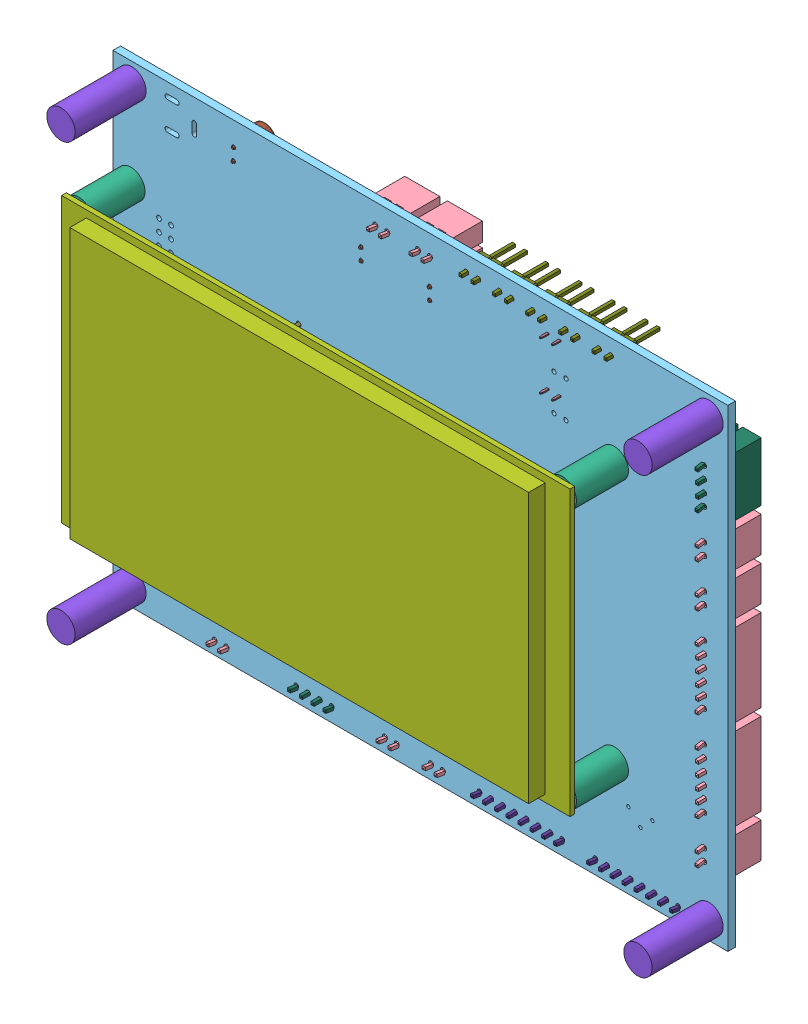
SolidWorks assembly MCU, configuration 默认. Lengths in mm. (continued)
Components (placement in the parent): (continued)
- MCU(2)^MCU-1: MCU(2)^MCU [默认] at origin size (130 100 11.94) (virtual) (continued)
  - R_0805^MCU(2)_MCU-76: R_0805^MCU(2)_MCU [默认] at (107.6 84.5 -0.05) x (1 0 0) z (0 0 -1) size (2 1.25 0.5) (virtual)
    - SOLID-1^R_0805_MCU(2)_MCU-1: SOLID-1^R_0805_MCU(2)_MCU [默认] at origin size (2 1.25 0.5) (virtual)
  - R_0805^MCU(2)_MCU-77: R_0805^MCU(2)_MCU [默认] at (120 86.5 -0.05) x (-1 0 0) z (0 0 -1) size (2 1.25 0.5) (virtual)
    - SOLID-1^R_0805_MCU(2)_MCU-1: SOLID-1^R_0805_MCU(2)_MCU [默认] at origin size (2 1.25 0.5) (virtual)
  - R_0805^MCU(2)_MCU-78: R_0805^MCU(2)_MCU [默认] at (51.9 8.7 -0.05) x (-1 0 0) z (0 0 -1) size (2 1.25 0.5) (virtual)
    - SOLID-1^R_0805_MCU(2)_MCU-1: SOLID-1^R_0805_MCU(2)_MCU [默认] at origin size (2 1.25 0.5) (virtual)
  - R_0805^MCU(2)_MCU-79: R_0805^MCU(2)_MCU [默认] at (46.929 55.357 -0.05) x (0.707107 0.707107 0) z (0 0 -1) size (2 1.25 0.5) (virtual)
    - SOLID-1^R_0805_MCU(2)_MCU-1: SOLID-1^R_0805_MCU(2)_MCU [默认] at origin size (2 1.25 0.5) (virtual)
  - R_0805^MCU(2)_MCU-80: R_0805^MCU(2)_MCU [默认] at (99.5 8.5 -0.05) x (-1 0 0) z (0 0 -1) size (2 1.25 0.5) (virtual)
    - SOLID-1^R_0805_MCU(2)_MCU-1: SOLID-1^R_0805_MCU(2)_MCU [默认] at origin size (2 1.25 0.5) (virtual)
  - R_0805^MCU(2)_MCU-81: R_0805^MCU(2)_MCU [默认] at (103.05 8.5 -0.05) x (-1 0 0) z (0 0 -1) size (2 1.25 0.5) (virtual)
    - SOLID-1^R_0805_MCU(2)_MCU-1: SOLID-1^R_0805_MCU(2)_MCU [默认] at origin size (2 1.25 0.5) (virtual)
  - R_0805^MCU(2)_MCU-82: R_0805^MCU(2)_MCU [默认] at (106.5 8.5 -0.05) x (1 0 0) z (0 0 -1) size (2 1.25 0.5) (virtual)
    - SOLID-1^R_0805_MCU(2)_MCU-1: SOLID-1^R_0805_MCU(2)_MCU [默认] at origin size (2 1.25 0.5) (virtual)
  - R_0805^MCU(2)_MCU-83: R_0805^MCU(2)_MCU [默认] at (110 8.5 -0.05) x (1 0 0) z (0 0 -1) size (2 1.25 0.5) (virtual)
    - SOLID-1^R_0805_MCU(2)_MCU-1: SOLID-1^R_0805_MCU(2)_MCU [默认] at origin size (2 1.25 0.5) (virtual)
  - R_0805^MCU(2)_MCU-84: R_0805^MCU(2)_MCU [默认] at (113.5 8.5 -0.05) x (-1 0 0) z (0 0 -1) size (2 1.25 0.5) (virtual)
    - SOLID-1^R_0805_MCU(2)_MCU-1: SOLID-1^R_0805_MCU(2)_MCU [默认] at origin size (2 1.25 0.5) (virtual)
  - R_0805^MCU(2)_MCU-85: R_0805^MCU(2)_MCU [默认] at (117 8.5 -0.05) x (-1 0 0) z (0 0 -1) size (2 1.25 0.5) (virtual)
    - SOLID-1^R_0805_MCU(2)_MCU-1: SOLID-1^R_0805_MCU(2)_MCU [默认] at origin size (2 1.25 0.5) (virtual)
  - R_0805^MCU(2)_MCU-86: R_0805^MCU(2)_MCU [默认] at (76.5 8.5 -0.05) x (1 0 0) z (0 0 -1) size (2 1.25 0.5) (virtual)
    - SOLID-1^R_0805_MCU(2)_MCU-1: SOLID-1^R_0805_MCU(2)_MCU [默认] at origin size (2 1.25 0.5) (virtual)
  - R_0805^MCU(2)_MCU-87: R_0805^MCU(2)_MCU [默认] at (80 8.5 -0.05) x (1 0 0) z (0 0 -1) size (2 1.25 0.5) (virtual)
    - SOLID-1^R_0805_MCU(2)_MCU-1: SOLID-1^R_0805_MCU(2)_MCU [默认] at origin size (2 1.25 0.5) (virtual)
  - R_0805^MCU(2)_MCU-88: R_0805^MCU(2)_MCU [默认] at (83.5 8.5 -0.05) x (1 0 0) z (0 0 -1) size (2 1.25 0.5) (virtual)
    - SOLID-1^R_0805_MCU(2)_MCU-1: SOLID-1^R_0805_MCU(2)_MCU [默认] at origin size (2 1.25 0.5) (virtual)
  - R_0805^MCU(2)_MCU-89: R_0805^MCU(2)_MCU [默认] at (87 8.5 -0.05) x (1 0 0) z (0 0 -1) size (2 1.25 0.5) (virtual)
    - SOLID-1^R_0805_MCU(2)_MCU-1: SOLID-1^R_0805_MCU(2)_MCU [默认] at origin size (2 1.25 0.5) (virtual)
  - R_0805^MCU(2)_MCU-90: R_0805^MCU(2)_MCU [默认] at (90.5 8.5 -0.05) x (1 0 0) z (0 0 -1) size (2 1.25 0.5) (virtual)
    - SOLID-1^R_0805_MCU(2)_MCU-1: SOLID-1^R_0805_MCU(2)_MCU [默认] at origin size (2 1.25 0.5) (virtual)
  - R_0805^MCU(2)_MCU-91: R_0805^MCU(2)_MCU [默认] at (94 8.5 -0.05) x (1 0 0) z (0 0 -1) size (2 1.25 0.5) (virtual)
    - SOLID-1^R_0805_MCU(2)_MCU-1: SOLID-1^R_0805_MCU(2)_MCU [默认] at origin size (2 1.25 0.5) (virtual)
  - SOT-23^MCU(2)_MCU-4: SOT-23^MCU(2)_MCU [默认] at (95.75 58.25 -0.05) x (0 1 0) z (0 0 -1) size (2.5 3 1.2) (virtual)
    - SOLID-4^SOT-23_MCU(2)_MCU-1: SOLID-4^SOT-23_MCU(2)_MCU [默认] at origin size (2.5 3 1.2) (virtual)
  - SOT-23^MCU(2)_MCU-5: SOT-23^MCU(2)_MCU [默认] at (99.75 53.35 -0.05) x (0 -1 0) z (0 0 -1) size (2.5 3 1.2) (virtual)
    - SOLID-4^SOT-23_MCU(2)_MCU-1: SOLID-4^SOT-23_MCU(2)_MCU [默认] at origin size (2.5 3 1.2) (virtual)
  - SOT-23^MCU(2)_MCU-6: SOT-23^MCU(2)_MCU [默认] at (96.25 51.25 -0.05) x (0 1 0) z (0 0 -1) size (2.5 3 1.2) (virtual)
    - SOLID-4^SOT-23_MCU(2)_MCU-1: SOLID-4^SOT-23_MCU(2)_MCU [默认] at origin size (2.5 3 1.2) (virtual)
  - SOT-23^MCU(2)_MCU-7: SOT-23^MCU(2)_MCU [默认] at (90.25 85.25 -0.05) x (0 -1 0) z (0 0 -1) size (2.5 3 1.2) (virtual)
    - SOLID-4^SOT-23_MCU(2)_MCU-1: SOLID-4^SOT-23_MCU(2)_MCU [默认] at origin size (2.5 3 1.2) (virtual)
  - SOT-23^MCU(2)_MCU-8: SOT-23^MCU(2)_MCU [默认] at (67.35 24.616 -0.05) x (0 -1 0) z (0 0 -1) size (2.5 3 1.2) (virtual)
    - SOLID-4^SOT-23_MCU(2)_MCU-1: SOLID-4^SOT-23_MCU(2)_MCU [默认] at origin size (2.5 3 1.2) (virtual)
  - SOT-23^MCU(2)_MCU-9: SOT-23^MCU(2)_MCU [默认] at (69.4 8.949 -0.05) x (0 -1 0) z (0 0 -1) size (2.5 3 1.2) (virtual)
    - SOLID-4^SOT-23_MCU(2)_MCU-1: SOLID-4^SOT-23_MCU(2)_MCU [默认] at origin size (2.5 3 1.2) (virtual)
  - SOT-23^MCU(2)_MCU-10: SOT-23^MCU(2)_MCU [默认] at (61.35 12.85 -0.05) x (0 -1 0) z (0 0 -1) size (2.5 3 1.2) (virtual)
    - SOLID-4^SOT-23_MCU(2)_MCU-1: SOLID-4^SOT-23_MCU(2)_MCU [默认] at origin size (2.5 3 1.2) (virtual)
  - SOT-23^MCU(2)_MCU-11: SOT-23^MCU(2)_MCU [默认] at (51.9 3.5 -0.05) x (0 -1 0) z (0 0 -1) size (2.5 3 1.2) (virtual)
    - SOLID-4^SOT-23_MCU(2)_MCU-1: SOLID-4^SOT-23_MCU(2)_MCU [默认] at origin size (2.5 3 1.2) (virtual)
  - L_1206^MCU(2)_MCU-1: L_1206^MCU(2)_MCU [默认] at (21 93 -0.05) x (0 1 0) z (0 0 -1) size (3.2 1.6 0.85) (virtual)
    - SOLID-18^L_1206_MCU(2)_MCU-1: SOLID-18^L_1206_MCU(2)_MCU [默认] at origin size (3.2 1.6 0.85) (virtual)
  - L_0805^MCU(2)_MCU-1: L_0805^MCU(2)_MCU [默认] at (23.053 67.93 -0.05) x (1 0 0) z (0 0 -1) size (2 1.25 1.25) (virtual)
    - SOLID-19^L_0805_MCU(2)_MCU-1: SOLID-19^L_0805_MCU(2)_MCU [默认] at origin size (2 1.25 1.25) (virtual)
  - L_0805^MCU(2)_MCU-2: L_0805^MCU(2)_MCU [默认] at (23.18 65.136 -0.05) x (1 0 0) z (0 0 -1) size (2 1.25 1.25) (virtual)
    - SOLID-19^L_0805_MCU(2)_MCU-1: SOLID-19^L_0805_MCU(2)_MCU [默认] at origin size (2 1.25 1.25) (virtual)
  - L_0805^MCU(2)_MCU-3: L_0805^MCU(2)_MCU [默认] at (34.0118 36.4708 -0.05) x (0.707107 0.707107 0) z (0 0 -1) size (2 1.25 1.25) (virtual)
    - SOLID-19^L_0805_MCU(2)_MCU-1: SOLID-19^L_0805_MCU(2)_MCU [默认] at origin size (2 1.25 1.25) (virtual)
  - Pin_Header_Straight_1x02_Pitch2.54mm^MCU(2)_MCU-3: Pin_Header_Straight_1x02_Pitch2.54mm^MCU(2)_MCU [默认] at (102.75 96.75 -0.05) x (0 -1 0) z (0 0 -1) size (2.54 5.08 11.54) (virtual)
    - SOLID-14^Pin_Header_Straight_1x02_Pitch2.54mm_MCU(2)_MCU-1: SOLID-14^Pin_Header_Straight_1x02_Pitch2.54mm_MCU(2)_MCU [默认] at origin size (2.54 5.08 11.54) (virtual)
  - Pin_Header_Straight_1x02_Pitch2.54mm^MCU(2)_MCU-4: Pin_Header_Straight_1x02_Pitch2.54mm^MCU(2)_MCU [默认] at (84.25 96.75 -0.05) x (0 1 0) z (0 0 -1) size (2.54 5.08 11.54) (virtual)
    - SOLID-14^Pin_Header_Straight_1x02_Pitch2.54mm_MCU(2)_MCU-1: SOLID-14^Pin_Header_Straight_1x02_Pitch2.54mm_MCU(2)_MCU [默认] at origin size (2.54 5.08 11.54) (virtual)
  - Pin_Header_Straight_1x02_Pitch2.54mm^MCU(2)_MCU-5: Pin_Header_Straight_1x02_Pitch2.54mm^MCU(2)_MCU [默认] at (88.75 96.75 -0.05) x (0 -1 0) z (0 0 -1) size (2.54 5.08 11.54) (virtual)
    - SOLID-14^Pin_Header_Straight_1x02_Pitch2.54mm_MCU(2)_MCU-1: SOLID-14^Pin_Header_Straight_1x02_Pitch2.54mm_MCU(2)_MCU [默认] at origin size (2.54 5.08 11.54) (virtual)
  - JST_XH_B02B-XH-A_02x2.50mm_Straight^MCU(2)_MCU-5: JST_XH_B02B-XH-A_02x2.50mm_Straight^MCU(2)_MCU [默认] at (67.25 3 -0.05) x (1 0 0) z (0 0 -1) size (7.4 5.75 10.4) (virtual)
    - SOLID-2^JST_XH_B02B-XH-A_02x2.50mm_Straight_MCU(2)_MCU-1: SOLID-2^JST_XH_B02B-XH-A_02x2.50mm_Straight_MCU(2)_MCU [默认] at origin size (7.4 5.75 10.4) (virtual)
  - JST_XH_B02B-XH-A_02x2.50mm_Straight^MCU(2)_MCU-6: JST_XH_B02B-XH-A_02x2.50mm_Straight^MCU(2)_MCU [默认] at (125 16.5 -0.05) x (0 -1 0) z (0 0 -1) size (7.4 5.75 10.4) (virtual)
    - SOLID-2^JST_XH_B02B-XH-A_02x2.50mm_Straight_MCU(2)_MCU-1: SOLID-2^JST_XH_B02B-XH-A_02x2.50mm_Straight_MCU(2)_MCU [默认] at origin size (7.4 5.75 10.4) (virtual)
  - JST_XH_B06B-XH-A_06x2.50mm_Straight^MCU(2)_MCU-1: JST_XH_B06B-XH-A_06x2.50mm_Straight^MCU(2)_MCU [默认] at (125 35.5 -0.05) x (0 -1 0) z (0 0 -1) size (17.4 5.75 10.4) (virtual)
    - SOLID-20^JST_XH_B06B-XH-A_06x2.50mm_Straight_MCU(2)_MCU-1: SOLID-20^JST_XH_B06B-XH-A_06x2.50mm_Straight_MCU(2)_MCU [默认] at origin size (17.4 5.75 10.4) (virtual)
  - JST_XH_B06B-XH-A_06x2.50mm_Straight^MCU(2)_MCU-2: JST_XH_B06B-XH-A_06x2.50mm_Straight^MCU(2)_MCU [默认] at (125 54.5 -0.05) x (0 -1 0) z (0 0 -1) size (17.4 5.75 10.4) (virtual)
    - SOLID-20^JST_XH_B06B-XH-A_06x2.50mm_Straight_MCU(2)_MCU-1: SOLID-20^JST_XH_B06B-XH-A_06x2.50mm_Straight_MCU(2)_MCU [默认] at origin size (17.4 5.75 10.4) (virtual)
  - JST_XH_B02B-XH-A_02x2.50mm_Straight^MCU(2)_MCU-7: JST_XH_B02B-XH-A_02x2.50mm_Straight^MCU(2)_MCU [默认] at (125 63.5 -0.05) x (0 -1 0) z (0 0 -1) size (7.4 5.75 10.4) (virtual)
    - SOLID-2^JST_XH_B02B-XH-A_02x2.50mm_Straight_MCU(2)_MCU-1: SOLID-2^JST_XH_B02B-XH-A_02x2.50mm_Straight_MCU(2)_MCU [默认] at origin size (7.4 5.75 10.4) (virtual)
  - JST_XH_B02B-XH-A_02x2.50mm_Straight^MCU(2)_MCU-8: JST_XH_B02B-XH-A_02x2.50mm_Straight^MCU(2)_MCU [默认] at (125 72.5 -0.05) x (0 -1 0) z (0 0 -1) size (7.4 5.75 10.4) (virtual)
    - SOLID-2^JST_XH_B02B-XH-A_02x2.50mm_Straight_MCU(2)_MCU-1: SOLID-2^JST_XH_B02B-XH-A_02x2.50mm_Straight_MCU(2)_MCU [默认] at origin size (7.4 5.75 10.4) (virtual)
  - JST_XH_B04B-XH-A_04x2.50mm_Straight^MCU(2)_MCU-2: JST_XH_B04B-XH-A_04x2.50mm_Straight^MCU(2)_MCU [默认] at (125 86.5 -0.05) x (0 -1 0) z (0 0 -1) size (12.4 5.75 10.4) (virtual)
    - SOLID-13^JST_XH_B04B-XH-A_04x2.50mm_Straight_MCU(2)_MCU-1: SOLID-13^JST_XH_B04B-XH-A_04x2.50mm_Straight_MCU(2)_MCU [默认] at origin size (12.4 5.75 10.4) (virtual)
  - R_1206^MCU(2)_MCU-3: R_1206^MCU(2)_MCU [默认] at (17 88.75 -0.05) x (1 0 0) z (0 0 -1) size (3.2 1.6 0.55) (virtual)
    - SOLID-5^R_1206_MCU(2)_MCU-1: SOLID-5^R_1206_MCU(2)_MCU [默认] at origin size (3.2 1.6 0.55) (virtual)
  - C_0805^MCU(2)_MCU-13: C_0805^MCU(2)_MCU [默认] at (3.5 88.75 -0.05) x (0 1 0) z (0 0 -1) size (2 1.25 0.78) (virtual)
    - SOLID-3^C_0805_MCU(2)_MCU-1: SOLID-3^C_0805_MCU(2)_MCU [默认] at origin size (2 1.25 0.78) (virtual)
  - C_0805^MCU(2)_MCU-14: C_0805^MCU(2)_MCU [默认] at (38 95 -0.05) x (0 1 0) z (0 0 -1) size (2 1.25 0.78) (virtual)
    - SOLID-3^C_0805_MCU(2)_MCU-1: SOLID-3^C_0805_MCU(2)_MCU [默认] at origin size (2 1.25 0.78) (virtual)
  - C_0805^MCU(2)_MCU-15: C_0805^MCU(2)_MCU [默认] at (36 95 -0.05) x (0 1 0) z (0 0 -1) size (2 1.25 0.78) (virtual)
    - SOLID-3^C_0805_MCU(2)_MCU-1: SOLID-3^C_0805_MCU(2)_MCU [默认] at origin size (2 1.25 0.78) (virtual)
  - C_0805^MCU(2)_MCU-16: C_0805^MCU(2)_MCU [默认] at (32 91.5 -0.05) x (1 0 0) z (0 0 -1) size (2 1.25 0.78) (virtual)
    - SOLID-3^C_0805_MCU(2)_MCU-1: SOLID-3^C_0805_MCU(2)_MCU [默认] at origin size (2 1.25 0.78) (virtual)
  - C_0805^MCU(2)_MCU-17: C_0805^MCU(2)_MCU [默认] at (28.25 88.25 -0.05) x (0 -1 0) z (0 0 -1) size (2 1.25 0.78) (virtual)
    - SOLID-3^C_0805_MCU(2)_MCU-1: SOLID-3^C_0805_MCU(2)_MCU [默认] at origin size (2 1.25 0.78) (virtual)
  - C_0805^MCU(2)_MCU-18: C_0805^MCU(2)_MCU [默认] at (109.5 96 -0.05) x (-1 0 0) z (0 0 -1) size (2 1.25 0.78) (virtual)
    - SOLID-3^C_0805_MCU(2)_MCU-1: SOLID-3^C_0805_MCU(2)_MCU [默认] at origin size (2 1.25 0.78) (virtual)
  - C_0805^MCU(2)_MCU-19: C_0805^MCU(2)_MCU [默认] at (100.75 57 -0.05) x (1 0 0) z (0 0 -1) size (2 1.25 0.78) (virtual)
    - SOLID-3^C_0805_MCU(2)_MCU-1: SOLID-3^C_0805_MCU(2)_MCU [默认] at origin size (2 1.25 0.78) (virtual)
  - C_0805^MCU(2)_MCU-20: C_0805^MCU(2)_MCU [默认] at (89.5 88.5 -0.05) x (1 0 0) z (0 0 -1) size (2 1.25 0.78) (virtual)
    - SOLID-3^C_0805_MCU(2)_MCU-1: SOLID-3^C_0805_MCU(2)_MCU [默认] at origin size (2 1.25 0.78) (virtual)
  - C_0805^MCU(2)_MCU-21: C_0805^MCU(2)_MCU [默认] at (64.35 13.85 -0.05) x (0 -1 0) z (0 0 -1) size (2 1.25 0.78) (virtual)
    - SOLID-3^C_0805_MCU(2)_MCU-1: SOLID-3^C_0805_MCU(2)_MCU [默认] at origin size (2 1.25 0.78) (virtual)
  - C_0805^MCU(2)_MCU-22: C_0805^MCU(2)_MCU [默认] at (96.25 91 -0.05) x (0 1 0) z (0 0 -1) size (2 1.25 0.78) (virtual)
    - SOLID-3^C_0805_MCU(2)_MCU-1: SOLID-3^C_0805_MCU(2)_MCU [默认] at origin size (2 1.25 0.78) (virtual)
  - C_0805^MCU(2)_MCU-23: C_0805^MCU(2)_MCU [默认] at (99.7 84.2 -0.05) x (-1 0 0) z (0 0 -1) size (2 1.25 0.78) (virtual)
    - SOLID-3^C_0805_MCU(2)_MCU-1: SOLID-3^C_0805_MCU(2)_MCU [默认] at origin size (2 1.25 0.78) (virtual)
  - C_0805^MCU(2)_MCU-24: C_0805^MCU(2)_MCU [默认] at (65.35 10.35 -0.05) x (-1 0 0) z (0 0 -1) size (2 1.25 0.78) (virtual)
    - SOLID-3^C_0805_MCU(2)_MCU-1: SOLID-3^C_0805_MCU(2)_MCU [默认] at origin size (2 1.25 0.78) (virtual)
  - C_0805^MCU(2)_MCU-25: C_0805^MCU(2)_MCU [默认] at (58.35 10.85 -0.05) x (0 -1 0) z (0 0 -1) size (2 1.25 0.78) (virtual)
    - SOLID-3^C_0805_MCU(2)_MCU-1: SOLID-3^C_0805_MCU(2)_MCU [默认] at origin size (2 1.25 0.78) (virtual)
  - C_0805^MCU(2)_MCU-26: C_0805^MCU(2)_MCU [默认] at (117 18.2 -0.05) x (0 -1 0) z (0 0 -1) size (2 1.25 0.78) (virtual)
    - SOLID-3^C_0805_MCU(2)_MCU-1: SOLID-3^C_0805_MCU(2)_MCU [默认] at origin size (2 1.25 0.78) (virtual)
  - C_0805^MCU(2)_MCU-27: C_0805^MCU(2)_MCU [默认] at (120 55 -0.05) x (1 0 0) z (0 0 -1) size (2 1.25 0.78) (virtual)
    - SOLID-3^C_0805_MCU(2)_MCU-1: SOLID-3^C_0805_MCU(2)_MCU [默认] at origin size (2 1.25 0.78) (virtual)
  - C_0805^MCU(2)_MCU-28: C_0805^MCU(2)_MCU [默认] at (120 51 -0.05) x (1 0 0) z (0 0 -1) size (2 1.25 0.78) (virtual)
    - SOLID-3^C_0805_MCU(2)_MCU-1: SOLID-3^C_0805_MCU(2)_MCU [默认] at origin size (2 1.25 0.78) (virtual)
  - C_0805^MCU(2)_MCU-29: C_0805^MCU(2)_MCU [默认] at (120 47 -0.05) x (1 0 0) z (0 0 -1) size (2 1.25 0.78) (virtual)
    - SOLID-3^C_0805_MCU(2)_MCU-1: SOLID-3^C_0805_MCU(2)_MCU [默认] at origin size (2 1.25 0.78) (virtual)
  - C_0805^MCU(2)_MCU-30: C_0805^MCU(2)_MCU [默认] at (120 43 -0.05) x (1 0 0) z (0 0 -1) size (2 1.25 0.78) (virtual)
    - SOLID-3^C_0805_MCU(2)_MCU-1: SOLID-3^C_0805_MCU(2)_MCU [默认] at origin size (2 1.25 0.78) (virtual)
  - C_0805^MCU(2)_MCU-31: C_0805^MCU(2)_MCU [默认] at (120 36.5 -0.05) x (1 0 0) z (0 0 -1) size (2 1.25 0.78) (virtual)
    - SOLID-3^C_0805_MCU(2)_MCU-1: SOLID-3^C_0805_MCU(2)_MCU [默认] at origin size (2 1.25 0.78) (virtual)
  - C_0805^MCU(2)_MCU-32: C_0805^MCU(2)_MCU [默认] at (120 32.5 -0.05) x (1 0 0) z (0 0 -1) size (2 1.25 0.78) (virtual)
    - SOLID-3^C_0805_MCU(2)_MCU-1: SOLID-3^C_0805_MCU(2)_MCU [默认] at origin size (2 1.25 0.78) (virtual)
  - C_0805^MCU(2)_MCU-33: C_0805^MCU(2)_MCU [默认] at (120 28.5 -0.05) x (1 0 0) z (0 0 -1) size (2 1.25 0.78) (virtual)
    - SOLID-3^C_0805_MCU(2)_MCU-1: SOLID-3^C_0805_MCU(2)_MCU [默认] at origin size (2 1.25 0.78) (virtual)
  - C_0805^MCU(2)_MCU-34: C_0805^MCU(2)_MCU [默认] at (120 24.5 -0.05) x (1 0 0) z (0 0 -1) size (2 1.25 0.78) (virtual)
    - SOLID-3^C_0805_MCU(2)_MCU-1: SOLID-3^C_0805_MCU(2)_MCU [默认] at origin size (2 1.25 0.78) (virtual)
  - C_0805^MCU(2)_MCU-35: C_0805^MCU(2)_MCU [默认] at (104.4 52.1 -0.05) x (1 0 0) z (0 0 -1) size (2 1.25 0.78) (virtual)
    - SOLID-3^C_0805_MCU(2)_MCU-1: SOLID-3^C_0805_MCU(2)_MCU [默认] at origin size (2 1.25 0.78) (virtual)
  - C_0805^MCU(2)_MCU-36: C_0805^MCU(2)_MCU [默认] at (106.9 28.8 -0.05) x (-1 0 0) z (0 0 -1) size (2 1.25 0.78) (virtual)
    - SOLID-3^C_0805_MCU(2)_MCU-1: SOLID-3^C_0805_MCU(2)_MCU [默认] at origin size (2 1.25 0.78) (virtual)
  - C_0805^MCU(2)_MCU-37: C_0805^MCU(2)_MCU [默认] at (108.5 39 -0.05) x (0 1 0) z (0 0 -1) size (2 1.25 0.78) (virtual)
    - SOLID-3^C_0805_MCU(2)_MCU-1: SOLID-3^C_0805_MCU(2)_MCU [默认] at origin size (2 1.25 0.78) (virtual)
  - C_0805^MCU(2)_MCU-38: C_0805^MCU(2)_MCU [默认] at (106.5 71.6 -0.05) x (-1 0 0) z (0 0 -1) size (2 1.25 0.78) (virtual)
    - SOLID-3^C_0805_MCU(2)_MCU-1: SOLID-3^C_0805_MCU(2)_MCU [默认] at origin size (2 1.25 0.78) (virtual)
  - C_0805^MCU(2)_MCU-39: C_0805^MCU(2)_MCU [默认] at (119.5 69 -0.05) x (1 0 0) z (0 0 -1) size (2 1.25 0.78) (virtual)
    - SOLID-3^C_0805_MCU(2)_MCU-1: SOLID-3^C_0805_MCU(2)_MCU [默认] at origin size (2 1.25 0.78) (virtual)
  - C_0805^MCU(2)_MCU-40: C_0805^MCU(2)_MCU [默认] at (120 62.75 -0.05) x (1 0 0) z (0 0 -1) size (2 1.25 0.78) (virtual)
    - SOLID-3^C_0805_MCU(2)_MCU-1: SOLID-3^C_0805_MCU(2)_MCU [默认] at origin size (2 1.25 0.78) (virtual)
  - C_0805^MCU(2)_MCU-41: C_0805^MCU(2)_MCU [默认] at (120 73 -0.05) x (1 0 0) z (0 0 -1) size (2 1.25 0.78) (virtual)
    - SOLID-3^C_0805_MCU(2)_MCU-1: SOLID-3^C_0805_MCU(2)_MCU [默认] at origin size (2 1.25 0.78) (virtual)
  - C_0805^MCU(2)_MCU-42: C_0805^MCU(2)_MCU [默认] at (120 84.5 -0.05) x (1 0 0) z (0 0 -1) size (2 1.25 0.78) (virtual)
    - SOLID-3^C_0805_MCU(2)_MCU-1: SOLID-3^C_0805_MCU(2)_MCU [默认] at origin size (2 1.25 0.78) (virtual)
  - C_0805^MCU(2)_MCU-43: C_0805^MCU(2)_MCU [默认] at (120 88.5 -0.05) x (1 0 0) z (0 0 -1) size (2 1.25 0.78) (virtual)
    - SOLID-3^C_0805_MCU(2)_MCU-1: SOLID-3^C_0805_MCU(2)_MCU [默认] at origin size (2 1.25 0.78) (virtual)
  - C_0805^MCU(2)_MCU-44: C_0805^MCU(2)_MCU [默认] at (106.5 65.6 -0.05) x (-1 0 0) z (0 0 -1) size (2 1.25 0.78) (virtual)
    - SOLID-3^C_0805_MCU(2)_MCU-1: SOLID-3^C_0805_MCU(2)_MCU [默认] at origin size (2 1.25 0.78) (virtual)
  - C_0805^MCU(2)_MCU-45: C_0805^MCU(2)_MCU [默认] at (107.6 82.25 -0.05) x (-1 0 0) z (0 0 -1) size (2 1.25 0.78) (virtual)
    - SOLID-3^C_0805_MCU(2)_MCU-1: SOLID-3^C_0805_MCU(2)_MCU [默认] at origin size (2 1.25 0.78) (virtual)
  - C_0805^MCU(2)_MCU-46: C_0805^MCU(2)_MCU [默认] at (51.9 6.7 -0.05) x (1 0 0) z (0 0 -1) size (2 1.25 0.78) (virtual)
    - SOLID-3^C_0805_MCU(2)_MCU-1: SOLID-3^C_0805_MCU(2)_MCU [默认] at origin size (2 1.25 0.78) (virtual)
  - C_0805^MCU(2)_MCU-47: C_0805^MCU(2)_MCU [默认] at (37.219 33.826 -0.05) x (0.707107 -0.707107 0) z (0 0 -1) size (2 1.25 0.78) (virtual)
    - SOLID-3^C_0805_MCU(2)_MCU-1: SOLID-3^C_0805_MCU(2)_MCU [默认] at origin size (2 1.25 0.78) (virtual)
  - C_0805^MCU(2)_MCU-48: C_0805^MCU(2)_MCU [默认] at (38.719 35.326 -0.05) x (0.707107 -0.707107 0) z (0 0 -1) size (2 1.25 0.78) (virtual)
    - SOLID-3^C_0805_MCU(2)_MCU-1: SOLID-3^C_0805_MCU(2)_MCU [默认] at origin size (2 1.25 0.78) (virtual)
  - C_0805^MCU(2)_MCU-49: C_0805^MCU(2)_MCU [默认] at (49.342 52.055 -0.05) x (0.707107 0.707107 0) z (0 0 -1) size (2 1.25 0.78) (virtual)
    - SOLID-3^C_0805_MCU(2)_MCU-1: SOLID-3^C_0805_MCU(2)_MCU [默认] at origin size (2 1.25 0.78) (virtual)
  - C_0805^MCU(2)_MCU-50: C_0805^MCU(2)_MCU [默认] at (42.116 38.723 -0.05) x (0.707107 -0.707107 0) z (0 0 -1) size (2 1.25 0.78) (virtual)
    - SOLID-3^C_0805_MCU(2)_MCU-1: SOLID-3^C_0805_MCU(2)_MCU [默认] at origin size (2 1.25 0.78) (virtual)
  - C_0805^MCU(2)_MCU-51: C_0805^MCU(2)_MCU [默认] at (22.799 48.499 -0.05) x (-0.707107 -0.707107 0) z (0 0 -1) size (2 1.25 0.78) (virtual)
    - SOLID-3^C_0805_MCU(2)_MCU-1: SOLID-3^C_0805_MCU(2)_MCU [默认] at origin size (2 1.25 0.78) (virtual)
  - C_0805^MCU(2)_MCU-52: C_0805^MCU(2)_MCU [默认] at (32 38.5 -0.05) x (-0.707107 -0.707107 0) z (0 0 -1) size (2 1.25 0.78) (virtual)
    - SOLID-3^C_0805_MCU(2)_MCU-1: SOLID-3^C_0805_MCU(2)_MCU [默认] at origin size (2 1.25 0.78) (virtual)
  - C_0805^MCU(2)_MCU-53: C_0805^MCU(2)_MCU [默认] at (48.65 44.4 -0.05) x (0.707107 -0.707107 0) z (0 0 -1) size (2 1.25 0.78) (virtual)
    - SOLID-3^C_0805_MCU(2)_MCU-1: SOLID-3^C_0805_MCU(2)_MCU [默认] at origin size (2 1.25 0.78) (virtual)
  - C_0805^MCU(2)_MCU-54: C_0805^MCU(2)_MCU [默认] at (36.007 63.104 -0.05) x (0.707107 0.707107 0) z (0 0 -1) size (2 1.25 0.78) (virtual)
    - SOLID-3^C_0805_MCU(2)_MCU-1: SOLID-3^C_0805_MCU(2)_MCU [默认] at origin size (2 1.25 0.78) (virtual)
  - C_0805^MCU(2)_MCU-55: C_0805^MCU(2)_MCU [默认] at (46 67 -0.05) x (-0.707107 0.707107 0) z (0 0 -1) size (2 1.25 0.78) (virtual)
    - SOLID-3^C_0805_MCU(2)_MCU-1: SOLID-3^C_0805_MCU(2)_MCU [默认] at origin size (2 1.25 0.78) (virtual)
  - C_0805^MCU(2)_MCU-56: C_0805^MCU(2)_MCU [默认] at (44.627 42.611 -0.05) x (0.707107 0.707107 0) z (0 0 -1) size (2 1.25 0.78) (virtual)
    - SOLID-3^C_0805_MCU(2)_MCU-1: SOLID-3^C_0805_MCU(2)_MCU [默认] at origin size (2 1.25 0.78) (virtual)
  - C_0805^MCU(2)_MCU-57: C_0805^MCU(2)_MCU [默认] at (48.834 38.72 -0.05) x (-0.707107 -0.707107 0) z (0 0 -1) size (2 1.25 0.78) (virtual)
    - SOLID-3^C_0805_MCU(2)_MCU-1: SOLID-3^C_0805_MCU(2)_MCU [默认] at origin size (2 1.25 0.78) (virtual)
  - 复件 COMPOUND^MCU(2)_MCU-1: 复件 COMPOUND^MCU(2)_MCU [默认] at origin size (130 100 1.6) (virtual)
- 零件24^MCU-1: 零件24^MCU [默认] at (0 0 1.6) size (108.2 61 11) (virtual)
- 零件25^MCU-1: 零件25^MCU [默认] at (0 0 12.6) size (107.5 60 4.5) (virtual)
- 零件26^MCU-1: 零件26^MCU [默认] at (0 0 1.6) size (128 98 15) (virtual)
Mates (geometry in assembly coordinates):
- 在位1: in place: plane of MCU(2)^MCU-1/复件 COMPOUND^MCU(2)_MCU-1 through (65 50 1.6) normal (0 0 1); plane of ? through (0 0 1.6) normal (0 0 1); moOrthogonalPlaneRef_w of MCU(2)^MCU-1/复件 COMPOUND^MCU(2)_MCU-1 through (65 50 1.6) normal (0 0 1); plane of ? through (0 0 1.6) normal (0 1 0); plane of MCU(2)^MCU-1/复件 COMPOUND^MCU(2)_MCU-1 through (65 50 1.6) normal (0 0 1); plane of ? through (0 0 1.6) normal (1 0 0); plane of MCU(2)^MCU-1/复件 COMPOUND^MCU(2)_MCU-1 through (65 50 1.6) normal (0 0 1); unknown of ?
- 重合1: coincident: plane of MCU(2)^MCU-1/复件 COMPOUND^MCU(2)_MCU-1; plane of 零件24^MCU-1
- 重合2: coincident: moOrthogonalPlaneRef_w of MCU(2)^MCU-1/复件 COMPOUND^MCU(2)_MCU-1 through (0 0 1.6) normal (0 1 0); plane of 零件24^MCU-1 through (0 0 1.6) normal (0 1 0)
- 重合3: coincident: moOrthogonalPlaneRef_w of MCU(2)^MCU-1/复件 COMPOUND^MCU(2)_MCU-1 through (0 0 1.6) normal (-1 0 0); plane of 零件24^MCU-1 through (0 0 1.6) normal (1 0 0)
- 在位2: in place: plane of ? through (3.775 22.5 12.6) normal (0 0 1); plane of 零件25^MCU-1 through (0 0 12.6) normal (0 0 1); plane of ? through (3.775 22.5 12.6) normal (0 0 1); plane of 零件25^MCU-1 through (0 0 12.6) normal (0 1 0); plane of ? through (3.775 22.5 12.6) normal (0 0 1); plane of 零件25^MCU-1 through (0 0 12.6) normal (1 0 0); plane of ? through (3.775 22.5 12.6) normal (0 0 1); unknown of 零件25^MCU-1
- 重合4: coincident: plane of 零件24^MCU-1; plane of 零件25^MCU-1
- 重合5: coincident: moOrthogonalPlaneRef_w of 零件24^MCU-1 through (0 0 12.6) normal (0 1 0); plane of 零件25^MCU-1 through (0 0 12.6) normal (0 1 0)
- 重合6: coincident: moOrthogonalPlaneRef_w of 零件24^MCU-1 through (0 0 12.6) normal (-1 0 0); plane of 零件25^MCU-1 through (0 0 12.6) normal (1 0 0)
- 在位3: in place: plane of MCU(2)^MCU-1/复件 COMPOUND^MCU(2)_MCU-1 through (65 50 1.6) normal (0 0 1); plane of ? through (0 0 1.6) normal (0 0 1); plane of MCU(2)^MCU-1/复件 COMPOUND^MCU(2)_MCU-1 through (65 50 1.6) normal (0 0 1); plane of ? through (0 0 1.6) normal (0 1 0); plane of MCU(2)^MCU-1/复件 COMPOUND^MCU(2)_MCU-1 through (65 50 1.6) normal (0 0 1); plane of ? through (0 0 1.6) normal (1 0 0); plane of MCU(2)^MCU-1/复件 COMPOUND^MCU(2)_MCU-1 through (65 50 1.6) normal (0 0 1); unknown of ?
- 重合7: coincident: plane of MCU(2)^MCU-1/复件 COMPOUND^MCU(2)_MCU-1; plane of 零件26^MCU-1
- 重合8: coincident: moOrthogonalPlaneRef_w of MCU(2)^MCU-1/复件 COMPOUND^MCU(2)_MCU-1 through (0 0 1.6) normal (0 1 0); plane of 零件26^MCU-1 through (0 0 1.6) normal (0 1 0)
- 重合9: coincident: moOrthogonalPlaneRef_w of MCU(2)^MCU-1/复件 COMPOUND^MCU(2)_MCU-1 through (0 0 1.6) normal (-1 0 0); plane of 零件26^MCU-1 through (0 0 1.6) normal (1 0 0)
